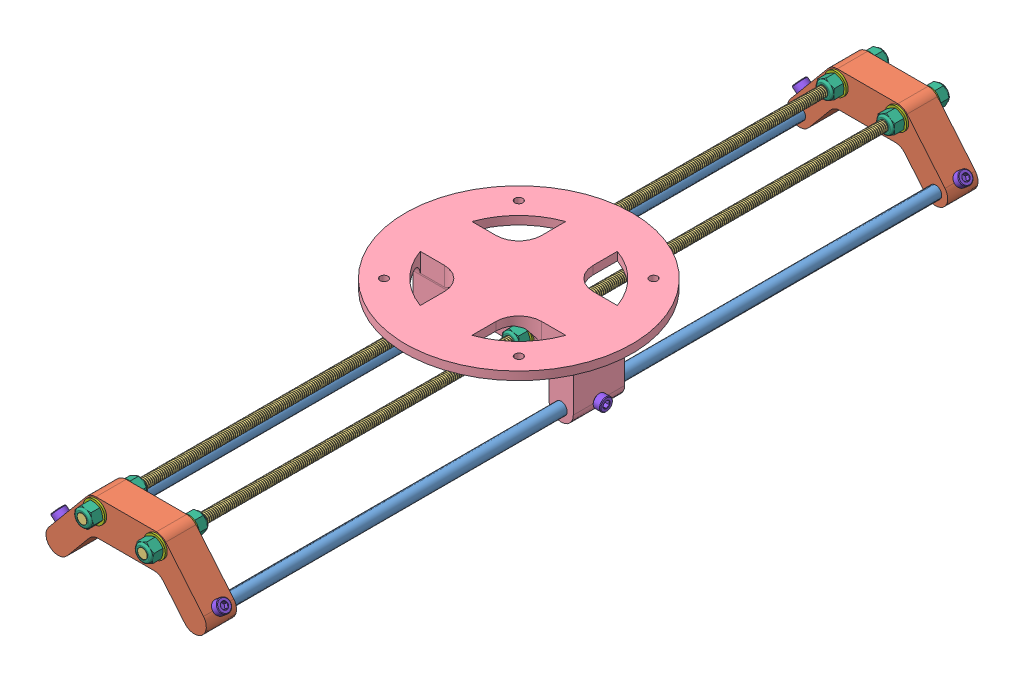
SolidWorks assembly X_Rail_Assembly, configuration Default. Lengths in mm.
Overall size (150 51.26 546.63).
43 component instances, 8 part files, 53 mates.
Components (placement in the parent):
- X_Rails-1: X_Rails [Default] at (161.7868 189.4775 32.4226) x (0.890472 0.455038 0) z (0 0 1) size (8 8 500)
- X_Rails-2: X_Rails [Default] at (71.7868 189.4775 32.4226) size (8 8 500)
- Rod_Endcaps-3: Rod_Endcaps [Default] at (116.7868 189.4775 27.4226) size (106 46 20)
- Rod_Endcaps-4: Rod_Endcaps [Default] at (116.7868 189.4775 537.4226) x (-1 0 0) z (0 0 -1) size (106 46 20)
- 0.25-20_Threaded_Rods-1: 0.25-20_Threaded_Rods [Default] at (136.7475 219.6116 18.2151) size (6.39 7.33 531.98)
- 0.25-20_Threaded_Rods-2: 0.25-20_Threaded_Rods [Default] at (96.8063 219.4522 18.2151) size (6.39 7.33 531.98)
- Center_Brace_Mount-1: Center_Brace_Mount [Default] at (116.7868 189.4775 260.9226) size (150 51.26 150)
- Threaded_Rod_Nuts-4: Threaded_Rod_Nuts [95462A029] at (136.7868 219.4775 277.4226) size (11.11 12.83 7.14)
- Threaded_Rod_Nuts-5: Threaded_Rod_Nuts [95462A029] at (96.7868 219.4775 277.4226) size (11.11 12.83 7.14)
- Endcap_Nut_Assem-1: Endcap_Nut_Assem [Default] at (183.8668 246.7356 56.1216) x (1 0 0) z (0 -1 0) size (16.57 38.42 16.57)
  - Nylock_0.25-20_Nut-1: Nylock_0.25-20_Nut [91831A029] at (-47.0799 -7.429 27.2581) size (11.11 8.13 12.83)
  - 0.24-20_Washer-1: 0.24-20_Washer [92916A365] at (-47.0799 -8.699 27.2581) x (0 1 0) z (-0.176891 0 0.984231) size (1.27 14.27 14.27)
  - 0.24-20_Washer-2: 0.24-20_Washer [92916A365] at (-47.0799 -28.699 27.2581) x (0 -1 0) z (-0.13862 0 0.990346) size (1.27 14.27 14.27)
  - Nylock_0.25-20_Nut-2: Nylock_0.25-20_Nut [91831A029] at (-47.0799 -29.969 27.2581) x (-0.911961 0 -0.410278) z (-0.410278 0 0.911961) size (11.11 8.13 12.83)
- Endcap_Nut_Assem-2: Endcap_Nut_Assem [Default] at (143.8668 246.7356 56.1216) x (1 0 0) z (0 -1 0) size (16.57 38.42 16.57)
  - Nylock_0.25-20_Nut-1: Nylock_0.25-20_Nut [91831A029] at (-47.0799 -7.429 27.2581) size (11.11 8.13 12.83)
  - 0.24-20_Washer-1: 0.24-20_Washer [92916A365] at (-47.0799 -8.699 27.2581) x (0 1 0) z (-0.176891 0 0.984231) size (1.27 14.27 14.27)
  - 0.24-20_Washer-2: 0.24-20_Washer [92916A365] at (-47.0799 -28.699 27.2581) x (0 -1 0) z (-0.13862 0 0.990346) size (1.27 14.27 14.27)
  - Nylock_0.25-20_Nut-2: Nylock_0.25-20_Nut [91831A029] at (-47.0799 -29.969 27.2581) x (-0.911961 0 -0.410278) z (-0.410278 0 0.911961) size (11.11 8.13 12.83)
- Endcap_Nut_Assem-3: Endcap_Nut_Assem [Default] at (132.9182 260.1475 546.1216) x (0.949358 0.314196 0) z (0.314196 -0.949358 0) size (16.57 38.42 16.57)
  - Nylock_0.25-20_Nut-1: Nylock_0.25-20_Nut [91831A029] at (-47.0799 -7.429 27.2581) size (11.11 8.13 12.83)
  - 0.24-20_Washer-1: 0.24-20_Washer [92916A365] at (-47.0799 -8.699 27.2581) x (0 1 0) z (-0.176891 0 0.984231) size (1.27 14.27 14.27)
  - 0.24-20_Washer-2: 0.24-20_Washer [92916A365] at (-47.0799 -28.699 27.2581) x (0 -1 0) z (-0.13862 0 0.990346) size (1.27 14.27 14.27)
  - Nylock_0.25-20_Nut-2: Nylock_0.25-20_Nut [91831A029] at (-47.0799 -29.969 27.2581) x (-0.911961 0 -0.410278) z (-0.410278 0 0.911961) size (11.11 8.13 12.83)
- Endcap_Nut_Assem-4: Endcap_Nut_Assem [Default] at (187.3914 239.4451 546.1216) x (0.988921 -0.14844 0) z (-0.14844 -0.988921 0) size (16.57 38.42 16.57)
  - Nylock_0.25-20_Nut-1: Nylock_0.25-20_Nut [91831A029] at (-47.0799 -7.429 27.2581) size (11.11 8.13 12.83)
  - 0.24-20_Washer-1: 0.24-20_Washer [92916A365] at (-47.0799 -8.699 27.2581) x (0 1 0) z (-0.176891 0 0.984231) size (1.27 14.27 14.27)
  - 0.24-20_Washer-2: 0.24-20_Washer [92916A365] at (-47.0799 -28.699 27.2581) x (0 -1 0) z (-0.13862 0 0.990346) size (1.27 14.27 14.27)
  - Nylock_0.25-20_Nut-2: Nylock_0.25-20_Nut [91831A029] at (-47.0799 -29.969 27.2581) x (-0.911961 0 -0.410278) z (-0.410278 0 0.911961) size (11.11 8.13 12.83)
- 0.24-20_Washer-1: 0.24-20_Washer [92916A365] at (96.7868 219.4775 294.9226) x (0 0 1) z (-0.999297 -0.037478 0) size (1.27 14.27 14.27)
- 0.24-20_Washer-2: 0.24-20_Washer [92916A365] at (96.7868 219.4775 259.6526) x (0 0 1) z (-1 0 0) size (1.27 14.27 14.27)
- 0.24-20_Washer-3: 0.24-20_Washer [92916A365] at (136.7868 219.4775 260.9226) x (0 0 -1) z (1 0 0) size (1.27 14.27 14.27)
- 0.24-20_Washer-4: 0.24-20_Washer [92916A365] at (136.7868 219.4775 296.1926) x (0 0 -1) z (0.999564 -0.02952 0) size (1.27 14.27 14.27)
- Nylock_0.25-20_Nut-1: Nylock_0.25-20_Nut [91831A029] at (136.7868 219.4775 259.6526) x (0.532067 -0.846702 0) z (0.846702 0.532067 0) size (11.11 8.13 12.83)
- Nylock_0.25-20_Nut-2: Nylock_0.25-20_Nut [91831A029] at (96.7868 219.4775 296.1926) x (1 0 0) z (0 -1 0) size (11.11 8.13 12.83)
- Nylock_0.25-20_Nut-3: Nylock_0.25-20_Nut [91831A029] at (136.7868 219.4775 296.1926) x (0.956813 0.290704 0) z (0.290704 -0.956813 0) size (11.11 8.13 12.83)
- Nylock_0.25-20_Nut-4: Nylock_0.25-20_Nut [91831A029] at (96.7868 219.4775 259.6526) x (0.999795 -0.020256 0) z (0.020256 0.999795 0) size (11.11 8.13 12.83)
- 8mm_M5x0-8_Bolt-1: 8mm_M5x0-8_Bolt [91292A191] at (161.7868 189.4775 527.4226) x (0.409836 -0.491803 0.768221) z (-0.768221 -0.640184 0) size (8.5 8.5 13.93)
- 8mm_M5x0-8_Bolt-2: 8mm_M5x0-8_Bolt [91292A191] at (71.7868 189.4775 527.4226) x (0.407117 0.48854 -0.771742) z (0.768221 -0.640184 0) size (8.5 8.5 13.93)
- 8mm_M5x0-8_Bolt-3: 8mm_M5x0-8_Bolt [91292A191] at (71.7868 189.4775 37.4226) x (0.407371 0.488845 -0.771414) z (0.768221 -0.640184 0) size (8.5 8.5 13.93)
- 8mm_M5x0-8_Bolt-4: 8mm_M5x0-8_Bolt [91292A191] at (161.7868 189.4775 37.4226) x (0.409836 -0.491803 0.768221) z (-0.768221 -0.640184 0) size (8.5 8.5 13.93)
- 8mm_M5x0-8_Bolt-5: 8mm_M5x0-8_Bolt [91292A191] at (161.7868 189.4775 277.9226) x (0 0 1) z (-1 0 0) size (8.5 8.5 13.93)
- 8mm_M5x0-8_Bolt-6: 8mm_M5x0-8_Bolt [91292A191] at (71.7868 189.4775 277.9226) x (0 0 -1) z (1 0 0) size (8.5 8.5 13.93)
Mates (geometry in assembly coordinates):
- Concentric1: concentric aligned: circle of X_Rails-2
- Concentric4: concentric anti-aligned: circle of X_Rails-1
- Parallel2: parallel aligned: plane of X_Rails-1 through (161.7868 189.4775 532.4226) normal (0 0 1); plane of X_Rails-2 through (71.7868 189.4775 532.4226) normal (0 0 1)
- Coincident2: coincident aligned: plane of X_Rails-1 through (161.7868 189.4775 532.4226) normal (0 0 1); plane of X_Rails-2 through (71.7868 189.4775 532.4226) normal (0 0 1)
- Concentric17: concentric aligned: circle of X_Rails-2; circle of Rod_Endcaps-3
- Concentric21: concentric aligned: circle of X_Rails-1; circle of Rod_Endcaps-3
- Coincident9: coincident anti-aligned: plane of X_Rails-2 through (71.7868 189.4775 32.4226) normal (0 0 -1); plane of Rod_Endcaps-3 through (71.7868 189.4775 32.4226) normal (0 0 1)
- Concentric22: concentric anti-aligned: circle of X_Rails-1; circle of Rod_Endcaps-4
- Concentric23: concentric anti-aligned: cone of X_Rails-2 through (71.7868 189.4775 532.4226) axis (0 0 1); circle of Rod_Endcaps-4
- Coincident10: coincident anti-aligned: plane of X_Rails-1 through (161.7868 189.4775 532.4226) normal (0 0 1); plane of Rod_Endcaps-4 through (161.7868 189.4775 532.4226) normal (0 0 -1)
- Distance1: distance = 9.2075 mm aligned: plane of Rod_Endcaps-3 through (96.7868 219.4775 27.4226) normal (0 0 -1); plane of 0.25-20_Threaded_Rods-1 through (136.7475 219.6116 18.2151) normal (0 0 -1)
- Coincident11: coincident aligned: plane of 0.25-20_Threaded_Rods-1 through (136.7475 219.6116 18.2151) normal (0 0 -1); plane of 0.25-20_Threaded_Rods-2 through (96.8063 219.4522 18.2151) normal (0 0 -1)
- Concentric30: concentric anti-aligned: circle of Rod_Endcaps-4; circle of Center_Brace_Mount-1
- Distance2: distance = 237.5 mm aligned: plane of Center_Brace_Mount-1 through (151.2868 208.7352 294.9226) normal (0 0 1); plane of X_Rails-2 through (71.7868 189.4775 532.4226) normal (0 0 1)
- Concentric33: concentric aligned: circle of Rod_Endcaps-4; circle of Center_Brace_Mount-1
- Concentric36: concentric aligned: circle of Rod_Endcaps-3; circle of Threaded_Rod_Nuts-4
- Concentric37: concentric anti-aligned: circle of Rod_Endcaps-3; circle of Threaded_Rod_Nuts-5
- Concentric56: concentric anti-aligned: circle of Rod_Endcaps-3; circle of Endcap_Nut_Assem-1/0.24-20_Washer-2
- Coincident36: coincident anti-aligned: plane of Rod_Endcaps-3 through (96.7868 219.4775 27.4226) normal (0 0 -1); plane of Endcap_Nut_Assem-1/0.24-20_Washer-2 through (136.7868 219.4775 27.4226) normal (0 0 1)
- Concentric58: concentric anti-aligned: circle of Rod_Endcaps-3; circle of Endcap_Nut_Assem-2/0.24-20_Washer-2
- Coincident37: coincident anti-aligned: plane of Rod_Endcaps-3 through (96.7868 219.4775 27.4226) normal (0 0 -1); plane of Endcap_Nut_Assem-2/0.24-20_Washer-2 through (96.7868 219.4775 27.4226) normal (0 0 1)
- Concentric59: concentric anti-aligned: circle of Rod_Endcaps-4; circle of Endcap_Nut_Assem-3/0.24-20_Washer-1
- Coincident38: coincident anti-aligned: plane of Rod_Endcaps-4 through (136.7868 219.4775 537.4226) normal (0 0 1); plane of Endcap_Nut_Assem-3/0.24-20_Washer-1 through (96.7868 219.4775 537.4226) normal (0 0 -1)
- Concentric60: concentric anti-aligned: circle of Rod_Endcaps-4; circle of Endcap_Nut_Assem-4/0.24-20_Washer-1
- Coincident39: coincident anti-aligned: plane of Rod_Endcaps-4 through (136.7868 219.4775 537.4226) normal (0 0 1); plane of Endcap_Nut_Assem-4/0.24-20_Washer-1 through (136.7868 219.4775 537.4226) normal (0 0 -1)
- Concentric61: concentric anti-aligned: circle of Center_Brace_Mount-1; circle of 0.24-20_Washer-1
- Coincident40: coincident anti-aligned: plane of Center_Brace_Mount-1 through (151.2868 208.7352 294.9226) normal (0 0 1); plane of 0.24-20_Washer-1 through (96.7868 219.4775 294.9226) normal (0 0 -1)
- Concentric62: concentric anti-aligned: circle of Center_Brace_Mount-1; circle of 0.24-20_Washer-2
- Coincident41: coincident anti-aligned: plane of Center_Brace_Mount-1 through (151.2868 208.7352 260.9226) normal (0 0 -1); plane of 0.24-20_Washer-2 through (96.7868 219.4775 260.9226) normal (0 0 1)
- Concentric63: concentric anti-aligned: circle of Center_Brace_Mount-1; circle of 0.24-20_Washer-3
- Coincident42: coincident anti-aligned: plane of Center_Brace_Mount-1 through (151.2868 208.7352 260.9226) normal (0 0 -1); plane of 0.24-20_Washer-3 through (136.7868 219.4775 260.9226) normal (0 0 1)
- Concentric64: concentric anti-aligned: circle of Center_Brace_Mount-1; circle of 0.24-20_Washer-4
- Coincident43: coincident anti-aligned: plane of Center_Brace_Mount-1 through (151.2868 208.7352 294.9226) normal (0 0 1); plane of 0.24-20_Washer-4 through (136.7868 219.4775 294.9226) normal (0 0 -1)
- Concentric65: concentric anti-aligned: circle of 0.24-20_Washer-4; circle of Nylock_0.25-20_Nut-1
- Coincident44: coincident anti-aligned: plane of 0.24-20_Washer-3 through (136.7868 219.4775 259.6526) normal (0 0 -1); plane of Nylock_0.25-20_Nut-1 through (125.6821 219.0615 259.6526) normal (0 0 1)
- Concentric66: concentric anti-aligned: circle of 0.24-20_Washer-1; circle of Nylock_0.25-20_Nut-2
- Coincident45: coincident anti-aligned: plane of 0.24-20_Washer-1 through (96.7868 219.4775 296.1926) normal (0 0 1); plane of Nylock_0.25-20_Nut-2 through (91.2306 229.1012 296.1926) normal (0 0 -1)
- Concentric68: concentric aligned: circle of 0.24-20_Washer-4; circle of Nylock_0.25-20_Nut-3
- Coincident46: coincident anti-aligned: plane of 0.24-20_Washer-4 through (136.7868 219.4775 296.1926) normal (0 0 1); plane of Nylock_0.25-20_Nut-3 through (128.6729 227.0703 296.1926) normal (0 0 -1)
- Concentric70: concentric aligned: circle of 0.24-20_Washer-2; circle of Nylock_0.25-20_Nut-4
- Coincident47: coincident anti-aligned: plane of 0.24-20_Washer-2 through (96.7868 219.4775 259.6526) normal (0 0 -1); plane of Nylock_0.25-20_Nut-4 through (91.0368 209.9683 259.6526) normal (0 0 1)
- Concentric71: concentric anti-aligned: circle of Rod_Endcaps-4; circle of 8mm_M5x0-8_Bolt-1
- Coincident48: coincident anti-aligned: plane of Rod_Endcaps-4 through (142.9326 224.599 517.4226) normal (0.768221 0.640184 0); plane of 8mm_M5x0-8_Bolt-1 through (167.9326 194.599 527.4226) normal (-0.768221 -0.640184 0)
- Concentric72: concentric anti-aligned: circle of Rod_Endcaps-4; circle of 8mm_M5x0-8_Bolt-2
- Coincident49: coincident anti-aligned: plane of Rod_Endcaps-4 through (90.6411 224.599 517.4226) normal (-0.768221 0.640184 0); plane of 8mm_M5x0-8_Bolt-2 through (65.6411 194.599 527.4226) normal (0.768221 -0.640184 0)
- Concentric73: concentric anti-aligned: circle of Rod_Endcaps-3; circle of 8mm_M5x0-8_Bolt-3
- Coincident50: coincident anti-aligned: plane of Rod_Endcaps-3 through (90.6411 224.599 47.4226) normal (-0.768221 0.640184 0); plane of 8mm_M5x0-8_Bolt-3 through (65.6411 194.599 37.4226) normal (0.768221 -0.640184 0)
- Concentric75: concentric anti-aligned: circle of Rod_Endcaps-3; circle of 8mm_M5x0-8_Bolt-4
- Coincident51: coincident anti-aligned: plane of Rod_Endcaps-3 through (142.9326 224.599 47.4226) normal (0.768221 0.640184 0); plane of 8mm_M5x0-8_Bolt-4 through (167.9326 194.599 37.4226) normal (-0.768221 -0.640184 0)
- Concentric76: concentric anti-aligned: circle of Center_Brace_Mount-1; circle of 8mm_M5x0-8_Bolt-5
- Coincident52: coincident anti-aligned: plane of Center_Brace_Mount-1 through (169.7868 227.2352 294.9226) normal (1 0 0); plane of 8mm_M5x0-8_Bolt-5 through (169.7868 189.4775 277.9226) normal (-1 0 0)
- Concentric77: concentric anti-aligned: circle of Center_Brace_Mount-1; circle of 8mm_M5x0-8_Bolt-6
- Coincident53: coincident anti-aligned: plane of Center_Brace_Mount-1 through (63.7868 207.2352 294.9226) normal (-1 0 0); plane of 8mm_M5x0-8_Bolt-6 through (63.7868 189.4775 277.9226) normal (1 0 0)
